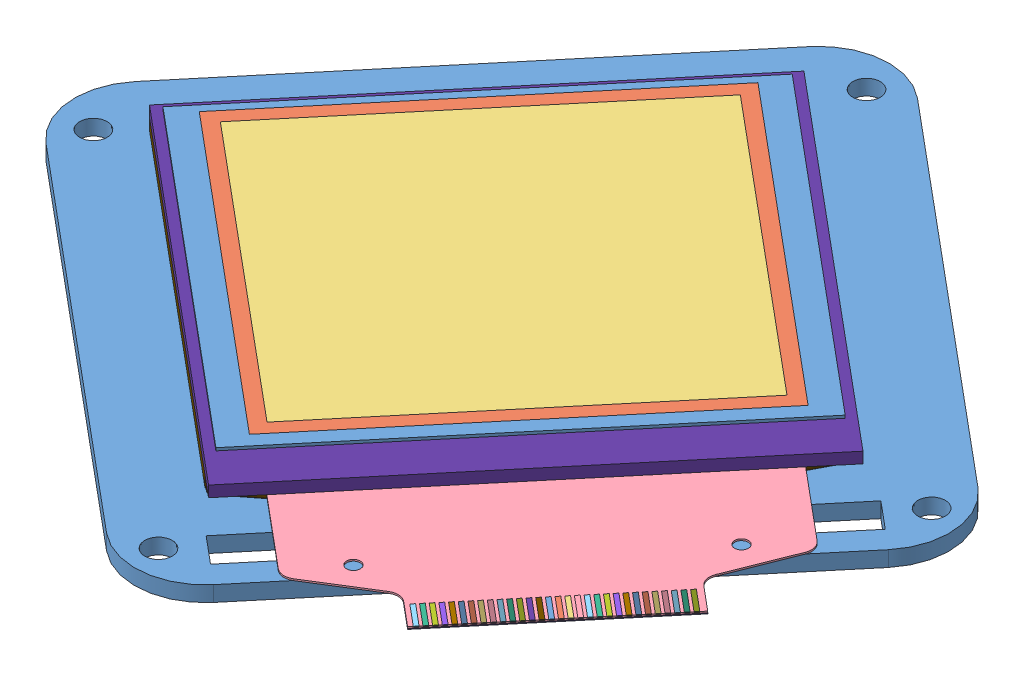
SolidWorks assembly main1, configuration 默认. Lengths in mm.
Overall size (158.53 67.75 132.39).
311 component instances, 75 part files, 5 mates.
Components (placement in the parent):
- case1-1: case1 [默认] at (23.4163 17.6612 38.5243) size (46 37.5 46)
- cubic1-1: cubic1 [默认] at (23.4663 19.1612 38.5743) x (0 0 1) z (-1 0 0) size (30 30 30)
- PCB_2020-12-27_16-28-50_2021-02-20_20-59-34-2: PCB_2020-12-27_16-28-50_2021-02-20_20-59-34 [默认] at (157.6255 16.5385 106.3075) x (-0.641097 0 0.76746) z (0 -1 0) size (45.01 51.47 7.58)
  - PCB_2020-12-27_16-28-50_2021-02-20_20-59-34.step-1: PCB_2020-12-27_16-28-50_2021-02-20_20-59-34.step [默认] at origin size (45.01 51.47 7.58)
    - Board.step-1: Board.step [默认] at origin size (45.01 45.01 1.12)
      - Open CASCADE STEP translator 6.8 3.1.1.step-1: Open CASCADE STEP translator 6.8 3.1.1.step [默认] at (0 0 -1.1227) size (45.01 45.01 1.12)
    - C34.step-1: C34.step [默认] at origin size (2.2 1.45 0.88)
      - c0805c101k5gactu.step-1: c0805c101k5gactu.step [默认] at (159.963 120.323 -10.6426) x (1 0 0) z (0 -1 0) size (2.2 0.88 1.45)
        - Open CASCADE STEP translator 6.8 3.2.1.1.step-1: Open CASCADE STEP translator 6.8 3.2.1.1.step [默认] at origin size (2 0.86 1.43)
        - Open CASCADE STEP translator 6.8 3.2.1.2.step-1: Open CASCADE STEP translator 6.8 3.2.1.2.step [默认] at origin size (0.34 0 0.18)
        - Open CASCADE STEP translator 6.8 3.2.1.3.step-1: Open CASCADE STEP translator 6.8 3.2.1.3.step [默认] at origin size (0.41 0 0.18)
        - Open CASCADE STEP translator 6.8 3.2.1.4.step-1: Open CASCADE STEP translator 6.8 3.2.1.4.step [默认] at origin size (0.21 0 0.18)
        - Open CASCADE STEP translator 6.8 3.2.1.5.step-1: Open CASCADE STEP translator 6.8 3.2.1.5.step [默认] at origin size (0.5 0.88 1.45)
        - Open CASCADE STEP translator 6.8 3.2.1.6.step-1: Open CASCADE STEP translator 6.8 3.2.1.6.step [默认] at origin size (0.5 0.88 1.45)
    - C14.step-1: C14.step [默认] at origin size (1.45 2.2 0.88)
      - c0805c101k5gactu.step-1: c0805c101k5gactu.step [默认] at (101.7169 -30.907 -10.6426) x (0 -1 0) z (-1 0 0) size (2.2 0.88 1.45)
        - Open CASCADE STEP translator 6.8 3.2.1.1.step-1: Open CASCADE STEP translator 6.8 3.2.1.1.step [默认] at origin size (2 0.86 1.43)
        - Open CASCADE STEP translator 6.8 3.2.1.2.step-1: Open CASCADE STEP translator 6.8 3.2.1.2.step [默认] at origin size (0.34 0 0.18)
        - Open CASCADE STEP translator 6.8 3.2.1.3.step-1: Open CASCADE STEP translator 6.8 3.2.1.3.step [默认] at origin size (0.41 0 0.18)
        - Open CASCADE STEP translator 6.8 3.2.1.4.step-1: Open CASCADE STEP translator 6.8 3.2.1.4.step [默认] at origin size (0.21 0 0.18)
        - Open CASCADE STEP translator 6.8 3.2.1.5.step-1: Open CASCADE STEP translator 6.8 3.2.1.5.step [默认] at origin size (0.5 0.88 1.45)
        - Open CASCADE STEP translator 6.8 3.2.1.6.step-1: Open CASCADE STEP translator 6.8 3.2.1.6.step [默认] at origin size (0.5 0.88 1.45)
    - C13.step-1: C13.step [默认] at origin size (0.95 1.77 0.95)
      - c0603x104k3ractu.step-1: c0603x104k3ractu.step [默认] at (16.3625 164.212 -10.6426) x (0 1 0) z (1 0 0) size (1.77 0.95 0.95)
        - Open CASCADE STEP translator 6.8 3.4.1.1.step-1: Open CASCADE STEP translator 6.8 3.4.1.1.step [默认] at origin size (1.57 0.93 0.93)
        - Open CASCADE STEP translator 6.8 3.4.1.2.step-1: Open CASCADE STEP translator 6.8 3.4.1.2.step [默认] at origin size (0.24 0 0.13)
        - Open CASCADE STEP translator 6.8 3.4.1.3.step-1: Open CASCADE STEP translator 6.8 3.4.1.3.step [默认] at origin size (0.29 0 0.13)
        - Open CASCADE STEP translator 6.8 3.4.1.4.step-1: Open CASCADE STEP translator 6.8 3.4.1.4.step [默认] at origin size (0.15 0 0.13)
        - Open CASCADE STEP translator 6.8 3.4.1.5.step-1: Open CASCADE STEP translator 6.8 3.4.1.5.step [默认] at origin size (0.45 0.95 0.95)
        - Open CASCADE STEP translator 6.8 3.4.1.6.step-1: Open CASCADE STEP translator 6.8 3.4.1.6.step [默认] at origin size (0.45 0.95 0.95)
    - C12.step-1: C12.step [默认] at origin size (0.95 1.77 0.95)
      - c0603x104k3ractu.step-1: c0603x104k3ractu.step [默认] at (9.3976 164.422 -10.6426) x (0 1 0) z (1 0 0) size (1.77 0.95 0.95)
        - Open CASCADE STEP translator 6.8 3.4.1.1.step-1: Open CASCADE STEP translator 6.8 3.4.1.1.step [默认] at origin size (1.57 0.93 0.93)
        - Open CASCADE STEP translator 6.8 3.4.1.2.step-1: Open CASCADE STEP translator 6.8 3.4.1.2.step [默认] at origin size (0.24 0 0.13)
        - Open CASCADE STEP translator 6.8 3.4.1.3.step-1: Open CASCADE STEP translator 6.8 3.4.1.3.step [默认] at origin size (0.29 0 0.13)
        - Open CASCADE STEP translator 6.8 3.4.1.4.step-1: Open CASCADE STEP translator 6.8 3.4.1.4.step [默认] at origin size (0.15 0 0.13)
        - Open CASCADE STEP translator 6.8 3.4.1.5.step-1: Open CASCADE STEP translator 6.8 3.4.1.5.step [默认] at origin size (0.45 0.95 0.95)
        - Open CASCADE STEP translator 6.8 3.4.1.6.step-1: Open CASCADE STEP translator 6.8 3.4.1.6.step [默认] at origin size (0.45 0.95 0.95)
    - USB2.step-1: USB2.step [默认] at origin size (5 7.8 2.7)
      - User_Library-micro_usb_SMD_RGB8421504.step-1: User_Library-micro_usb_SMD_RGB8421504.step [默认] at (44.3599 67.8551 1.27) x (0 -1 0) z (-1 0 0) size (7.8 2.7 5)
    - R7.step-1: R7.step [默认] at origin size (1.6 0.8 0.42)
      - User_Library-Res-0603.step-1: User_Library-Res-0603.step [默认] at (87.122 80.8989 0) x (-1 0 0) z (0 1 0) size (1.6 0.42 0.8)
    - L2.step-1: L2.step [默认] at origin size (0.86 1.6 0.51)
      - CircuitWorks-RESISTOR_0603.step-1: CircuitWorks-RESISTOR_0603.step [默认] at (61.595 79.7559 0) x (0 -1 0) z (-1 0 0) size (1.6 0.51 0.86)
    - P2.step-1: P2.step [默认] at origin size (20.43 5.11 2.05)
      - 3-1734839-0_RGB8421504.step-1: 3-1734839-0_RGB8421504.step [默认] at (66.548 57.4041 1.0414) x (1 0 0) z (0 -1 0) size (20.43 2.05 5.11)
    - D4.step-1: D4.step [默认] at origin size (3.7 1.6 1.27)
      - CircuitWorks-SOD123.step-1: CircuitWorks-SOD123.step [默认] at (72.4968 69.5129 0.0508) x (1 0 0) z (0 -1 0) size (3.7 1.27 1.6)
    - D5.step-1: D5.step [默认] at origin size (1.6 3.7 1.27)
      - CircuitWorks-SOD123.step-1: CircuitWorks-SOD123.step [默认] at (87.6301 64.8969 0.0508) x (0 1 0) z (1 0 0) size (3.7 1.27 1.6)
    - C21.step-1: C21.step [默认] at origin size (1.45 2.2 0.88)
      - c0805c101k5gactu.step-1: c0805c101k5gactu.step [默认] at (98.5419 -33.828 -10.6426) x (0 -1 0) z (-1 0 0) size (2.2 0.88 1.45)
        - Open CASCADE STEP translator 6.8 3.2.1.1.step-1: Open CASCADE STEP translator 6.8 3.2.1.1.step [默认] at origin size (2 0.86 1.43)
        - Open CASCADE STEP translator 6.8 3.2.1.2.step-1: Open CASCADE STEP translator 6.8 3.2.1.2.step [默认] at origin size (0.34 0 0.18)
        - Open CASCADE STEP translator 6.8 3.2.1.3.step-1: Open CASCADE STEP translator 6.8 3.2.1.3.step [默认] at origin size (0.41 0 0.18)
        - Open CASCADE STEP translator 6.8 3.2.1.4.step-1: Open CASCADE STEP translator 6.8 3.2.1.4.step [默认] at origin size (0.21 0 0.18)
        - Open CASCADE STEP translator 6.8 3.2.1.5.step-1: Open CASCADE STEP translator 6.8 3.2.1.5.step [默认] at origin size (0.5 0.88 1.45)
        - Open CASCADE STEP translator 6.8 3.2.1.6.step-1: Open CASCADE STEP translator 6.8 3.2.1.6.step [默认] at origin size (0.5 0.88 1.45)
    - C24.step-1: C24.step [默认] at origin size (1.45 2.2 0.88)
      - c0805c101k5gactu.step-1: c0805c101k5gactu.step [默认] at (2.51 156.471 -10.6426) x (0 1 0) z (1 0 0) size (2.2 0.88 1.45)
        - Open CASCADE STEP translator 6.8 3.2.1.1.step-1: Open CASCADE STEP translator 6.8 3.2.1.1.step [默认] at origin size (2 0.86 1.43)
        - Open CASCADE STEP translator 6.8 3.2.1.2.step-1: Open CASCADE STEP translator 6.8 3.2.1.2.step [默认] at origin size (0.34 0 0.18)
        - Open CASCADE STEP translator 6.8 3.2.1.3.step-1: Open CASCADE STEP translator 6.8 3.2.1.3.step [默认] at origin size (0.41 0 0.18)
        - Open CASCADE STEP translator 6.8 3.2.1.4.step-1: Open CASCADE STEP translator 6.8 3.2.1.4.step [默认] at origin size (0.21 0 0.18)
        - Open CASCADE STEP translator 6.8 3.2.1.5.step-1: Open CASCADE STEP translator 6.8 3.2.1.5.step [默认] at origin size (0.5 0.88 1.45)
        - Open CASCADE STEP translator 6.8 3.2.1.6.step-1: Open CASCADE STEP translator 6.8 3.2.1.6.step [默认] at origin size (0.5 0.88 1.45)
    - U7.step-1: U7.step [默认] at origin size (2.5 3 1.1)
      - CircuitWorks-SOT-23-5.step-1: CircuitWorks-SOT-23-5.step [默认] at (84.308 68.2431 -0.5131) x (0 1 0) z (1 0 0) size (3 1.1 2.5)
    - U5.step-1: U5.step [默认] at origin size (7 7 0.55)
      - User_Library-UFQFPN48.step-1: User_Library-UFQFPN48.step [默认] at (57.0029 73.1959 0) x (-1 0 0) z (0 0 1) size (7 7 0.55)
    - R13.step-1: R13.step [默认] at origin size (0.8 1.6 0.42)
      - User_Library-Res-0603.step-1: User_Library-Res-0603.step [默认] at (78.3388 65.957 0) x (0 1 0) z (1 0 0) size (1.6 0.42 0.8)
    - U4.step-1: U4.step [默认] at origin size (19.57 12.72 3.54)
      - User_Library-BK-885-TR.step-1: User_Library-BK-885-TR.step [默认] at (69.4691 84.328 0) x (1 0 0) z (0 -1 0) size (19.57 3.54 12.72)
    - U3.step-1: U3.step [默认] at origin size (0.8 1.6 0.42)
      - User_Library-Res-0603.step-1: User_Library-Res-0603.step [默认] at (61.3211 52.876 0) x (0 -1 0) z (-1 0 0) size (1.6 0.42 0.8)
    - C27.step-1: C27.step [默认] at origin size (0.95 1.77 0.95)
      - c0603x104k3ractu.step-1: c0603x104k3ractu.step [默认] at (123.9324 -30.647 -10.6426) x (0 -1 0) z (-1 0 0) size (1.77 0.95 0.95)
        - Open CASCADE STEP translator 6.8 3.4.1.1.step-1: Open CASCADE STEP translator 6.8 3.4.1.1.step [默认] at origin size (1.57 0.93 0.93)
        - Open CASCADE STEP translator 6.8 3.4.1.2.step-1: Open CASCADE STEP translator 6.8 3.4.1.2.step [默认] at origin size (0.24 0 0.13)
        - Open CASCADE STEP translator 6.8 3.4.1.3.step-1: Open CASCADE STEP translator 6.8 3.4.1.3.step [默认] at origin size (0.29 0 0.13)
        - Open CASCADE STEP translator 6.8 3.4.1.4.step-1: Open CASCADE STEP translator 6.8 3.4.1.4.step [默认] at origin size (0.15 0 0.13)
        - Open CASCADE STEP translator 6.8 3.4.1.5.step-1: Open CASCADE STEP translator 6.8 3.4.1.5.step [默认] at origin size (0.45 0.95 0.95)
        - Open CASCADE STEP translator 6.8 3.4.1.6.step-1: Open CASCADE STEP translator 6.8 3.4.1.6.step [默认] at origin size (0.45 0.95 0.95)
    - C20.step-1: C20.step [默认] at origin size (3.7 1.95 1.8)
      - c1206x223j2gacauto.step-1: c1206x223j2gacauto.step [默认] at (174.9253 96.5054 -10.6426) x (1 0 0) z (0 -1 0) size (3.7 1.8 1.95)
        - Open CASCADE STEP translator 6.8 3.20.1.1.step-1: Open CASCADE STEP translator 6.8 3.20.1.1.step [默认] at origin size (3.5 1.78 1.93)
        - Open CASCADE STEP translator 6.8 3.20.1.2.step-1: Open CASCADE STEP translator 6.8 3.20.1.2.step [默认] at origin size (0.7 0 0.37)
        - Open CASCADE STEP translator 6.8 3.20.1.3.step-1: Open CASCADE STEP translator 6.8 3.20.1.3.step [默认] at origin size (0.85 0 0.37)
        - Open CASCADE STEP translator 6.8 3.20.1.4.step-1: Open CASCADE STEP translator 6.8 3.20.1.4.step [默认] at origin size (0.44 0 0.37)
        - Open CASCADE STEP translator 6.8 3.20.1.5.step-1: Open CASCADE STEP translator 6.8 3.20.1.5.step [默认] at origin size (0.6 1.8 1.95)
        - Open CASCADE STEP translator 6.8 3.20.1.6.step-1: Open CASCADE STEP translator 6.8 3.20.1.6.step [默认] at origin size (0.6 1.8 1.95)
    - X3.step-1: X3.step [默认] at origin size (1.5 3.2 0.91)
      - crystal_rtf3215.step-1: crystal_rtf3215.step [默认] at (66.167 69.4691 0) x (0 1 0) z (1 0 0) size (3.2 0.91 1.5)
    - C28.step-1: C28.step [默认] at origin size (1.45 2.2 0.88)
      - c0805c101k5gactu.step-1: c0805c101k5gactu.step [默认] at (25.644 150.077 -10.6426) x (0 1 0) z (1 0 0) size (2.2 0.88 1.45)
        - Open CASCADE STEP translator 6.8 3.2.1.1.step-1: Open CASCADE STEP translator 6.8 3.2.1.1.step [默认] at origin size (2 0.86 1.43)
        - Open CASCADE STEP translator 6.8 3.2.1.2.step-1: Open CASCADE STEP translator 6.8 3.2.1.2.step [默认] at origin size (0.34 0 0.18)
        - Open CASCADE STEP translator 6.8 3.2.1.3.step-1: Open CASCADE STEP translator 6.8 3.2.1.3.step [默认] at origin size (0.41 0 0.18)
        - Open CASCADE STEP translator 6.8 3.2.1.4.step-1: Open CASCADE STEP translator 6.8 3.2.1.4.step [默认] at origin size (0.21 0 0.18)
        - Open CASCADE STEP translator 6.8 3.2.1.5.step-1: Open CASCADE STEP translator 6.8 3.2.1.5.step [默认] at origin size (0.5 0.88 1.45)
        - Open CASCADE STEP translator 6.8 3.2.1.6.step-1: Open CASCADE STEP translator 6.8 3.2.1.6.step [默认] at origin size (0.5 0.88 1.45)
    - C29.step-1: C29.step [默认] at origin size (1.45 2.2 0.88)
      - c0805c101k5gactu.step-1: c0805c101k5gactu.step [默认] at (102.7329 -43.6071 -10.6426) x (0 -1 0) z (-1 0 0) size (2.2 0.88 1.45)
        - Open CASCADE STEP translator 6.8 3.2.1.1.step-1: Open CASCADE STEP translator 6.8 3.2.1.1.step [默认] at origin size (2 0.86 1.43)
        - Open CASCADE STEP translator 6.8 3.2.1.2.step-1: Open CASCADE STEP translator 6.8 3.2.1.2.step [默认] at origin size (0.34 0 0.18)
        - Open CASCADE STEP translator 6.8 3.2.1.3.step-1: Open CASCADE STEP translator 6.8 3.2.1.3.step [默认] at origin size (0.41 0 0.18)
        - Open CASCADE STEP translator 6.8 3.2.1.4.step-1: Open CASCADE STEP translator 6.8 3.2.1.4.step [默认] at origin size (0.21 0 0.18)
        - Open CASCADE STEP translator 6.8 3.2.1.5.step-1: Open CASCADE STEP translator 6.8 3.2.1.5.step [默认] at origin size (0.5 0.88 1.45)
        - Open CASCADE STEP translator 6.8 3.2.1.6.step-1: Open CASCADE STEP translator 6.8 3.2.1.6.step [默认] at origin size (0.5 0.88 1.45)
    - C30.step-1: C30.step [默认] at origin size (1.45 2.2 0.88)
      - c0805c101k5gactu.step-1: c0805c101k5gactu.step [默认] at (97.9069 -43.6071 -10.6426) x (0 -1 0) z (-1 0 0) size (2.2 0.88 1.45)
        - Open CASCADE STEP translator 6.8 3.2.1.1.step-1: Open CASCADE STEP translator 6.8 3.2.1.1.step [默认] at origin size (2 0.86 1.43)
        - Open CASCADE STEP translator 6.8 3.2.1.2.step-1: Open CASCADE STEP translator 6.8 3.2.1.2.step [默认] at origin size (0.34 0 0.18)
        - Open CASCADE STEP translator 6.8 3.2.1.3.step-1: Open CASCADE STEP translator 6.8 3.2.1.3.step [默认] at origin size (0.41 0 0.18)
        - Open CASCADE STEP translator 6.8 3.2.1.4.step-1: Open CASCADE STEP translator 6.8 3.2.1.4.step [默认] at origin size (0.21 0 0.18)
        - Open CASCADE STEP translator 6.8 3.2.1.5.step-1: Open CASCADE STEP translator 6.8 3.2.1.5.step [默认] at origin size (0.5 0.88 1.45)
        - Open CASCADE STEP translator 6.8 3.2.1.6.step-1: Open CASCADE STEP translator 6.8 3.2.1.6.step [默认] at origin size (0.5 0.88 1.45)
    - U6.step-1: U6.step [默认] at origin size (2.5 3 1.1)
      - CircuitWorks-SOT-23-5.step-1: CircuitWorks-SOT-23-5.step [默认] at (52.8119 59.0989 -0.5131) x (0 -1 0) z (-1 0 0) size (3 1.1 2.5)
    - FPC1.step-1: FPC1.step [默认] at origin size (12.1 6.6 2)
      - 52746-1290_RGB10066329.step-1: 52746-1290_RGB10066329.step [默认] at (53.7211 87.5031 0) x (1 0 0) z (0 -1 0) size (12.1 2 6.6)
    - C18.step-1: C18.step [默认] at origin size (0.95 1.77 0.95)
      - c0603x104k3ractu.step-1: c0603x104k3ractu.step [默认] at (29.9716 149.69 -10.6426) x (0 1 0) z (1 0 0) size (1.77 0.95 0.95)
        - Open CASCADE STEP translator 6.8 3.4.1.1.step-1: Open CASCADE STEP translator 6.8 3.4.1.1.step [默认] at origin size (1.57 0.93 0.93)
        - Open CASCADE STEP translator 6.8 3.4.1.2.step-1: Open CASCADE STEP translator 6.8 3.4.1.2.step [默认] at origin size (0.24 0 0.13)
        - Open CASCADE STEP translator 6.8 3.4.1.3.step-1: Open CASCADE STEP translator 6.8 3.4.1.3.step [默认] at origin size (0.29 0 0.13)
        - Open CASCADE STEP translator 6.8 3.4.1.4.step-1: Open CASCADE STEP translator 6.8 3.4.1.4.step [默认] at origin size (0.15 0 0.13)
        - Open CASCADE STEP translator 6.8 3.4.1.5.step-1: Open CASCADE STEP translator 6.8 3.4.1.5.step [默认] at origin size (0.45 0.95 0.95)
        - Open CASCADE STEP translator 6.8 3.4.1.6.step-1: Open CASCADE STEP translator 6.8 3.4.1.6.step [默认] at origin size (0.45 0.95 0.95)
    - X1.step-1: X1.step [默认] at origin size (2.5 3.2 1.05)
      - User_Library-SMD-3225_4P.step-1: User_Library-SMD-3225_4P.step [默认] at (70.338 73.8309 0) x (0 -1 0) z (0 0 1) size (3.2 2.5 1.05)
    - C26.step-1: C26.step [默认] at origin size (2.2 1.45 0.88)
      - c0805c101k5gactu.step-1: c0805c101k5gactu.step [默认] at (183.605 114.818 -10.6426) x (1 0 0) z (0 -1 0) size (2.2 0.88 1.45)
        - Open CASCADE STEP translator 6.8 3.2.1.1.step-1: Open CASCADE STEP translator 6.8 3.2.1.1.step [默认] at origin size (2 0.86 1.43)
        - Open CASCADE STEP translator 6.8 3.2.1.2.step-1: Open CASCADE STEP translator 6.8 3.2.1.2.step [默认] at origin size (0.34 0 0.18)
        - Open CASCADE STEP translator 6.8 3.2.1.3.step-1: Open CASCADE STEP translator 6.8 3.2.1.3.step [默认] at origin size (0.41 0 0.18)
        - Open CASCADE STEP translator 6.8 3.2.1.4.step-1: Open CASCADE STEP translator 6.8 3.2.1.4.step [默认] at origin size (0.21 0 0.18)
        - Open CASCADE STEP translator 6.8 3.2.1.5.step-1: Open CASCADE STEP translator 6.8 3.2.1.5.step [默认] at origin size (0.5 0.88 1.45)
        - Open CASCADE STEP translator 6.8 3.2.1.6.step-1: Open CASCADE STEP translator 6.8 3.2.1.6.step [默认] at origin size (0.5 0.88 1.45)
    - C25.step-1: C25.step [默认] at origin size (1.45 2.2 0.88)
      - c0805c101k5gactu.step-1: c0805c101k5gactu.step [默认] at (36.439 156.681 -10.6426) x (0 1 0) z (1 0 0) size (2.2 0.88 1.45)
        - Open CASCADE STEP translator 6.8 3.2.1.1.step-1: Open CASCADE STEP translator 6.8 3.2.1.1.step [默认] at origin size (2 0.86 1.43)
        - Open CASCADE STEP translator 6.8 3.2.1.2.step-1: Open CASCADE STEP translator 6.8 3.2.1.2.step [默认] at origin size (0.34 0 0.18)
        - Open CASCADE STEP translator 6.8 3.2.1.3.step-1: Open CASCADE STEP translator 6.8 3.2.1.3.step [默认] at origin size (0.41 0 0.18)
        - Open CASCADE STEP translator 6.8 3.2.1.4.step-1: Open CASCADE STEP translator 6.8 3.2.1.4.step [默认] at origin size (0.21 0 0.18)
        - Open CASCADE STEP translator 6.8 3.2.1.5.step-1: Open CASCADE STEP translator 6.8 3.2.1.5.step [默认] at origin size (0.5 0.88 1.45)
        - Open CASCADE STEP translator 6.8 3.2.1.6.step-1: Open CASCADE STEP translator 6.8 3.2.1.6.step [默认] at origin size (0.5 0.88 1.45)
    - R17.step-1: R17.step [默认] at origin size (1.6 0.8 0.42)
      - User_Library-Res-0603.step-1: User_Library-Res-0603.step [默认] at (65.278 55.7531 0) x (1 0 0) z (0 -1 0) size (1.6 0.42 0.8)
    - R12.step-1: R12.step [默认] at origin size (0.8 1.6 0.42)
      - User_Library-Res-0603.step-1: User_Library-Res-0603.step [默认] at (63.2461 52.832 0) x (0 -1 0) z (-1 0 0) size (1.6 0.42 0.8)
    - R16.step-1: R16.step [默认] at origin size (1.6 0.8 0.42)
      - User_Library-Res-0603.step-1: User_Library-Res-0603.step [默认] at (62.103 55.7529 0) x (-1 0 0) z (0 1 0) size (1.6 0.42 0.8)
    - R15.step-1: R15.step [默认] at origin size (0.8 1.6 0.42)
      - User_Library-Res-0603.step-1: User_Library-Res-0603.step [默认] at (65.0241 52.832 0) x (0 -1 0) z (-1 0 0) size (1.6 0.42 0.8)
    - SW2.step-1: SW2.step [默认] at origin size (4.6 3.2 2.5)
      - skrpace010_RGB10066329.step-1: skrpace010_RGB10066329.step [默认] at (82.5499 81.661 0) x (-1 0 0) z (0 1 0) size (4.6 2.5 3.2)
    - SW1.step-1: SW1.step [默认] at origin size (4.6 3.2 2.5)
      - skrpace010_RGB10066329.step-1: skrpace010_RGB10066329.step [默认] at (82.4231 85.217 0) x (1 0 0) z (0 -1 0) size (4.6 2.5 3.2)
    - C17.step-1: C17.step [默认] at origin size (1.77 0.95 0.95)
      - c0603x104k3ractu.step-1: c0603x104k3ractu.step [默认] at (159.977 114.6814 -10.6426) x (1 0 0) z (0 -1 0) size (1.77 0.95 0.95)
        - Open CASCADE STEP translator 6.8 3.4.1.1.step-1: Open CASCADE STEP translator 6.8 3.4.1.1.step [默认] at origin size (1.57 0.93 0.93)
        - Open CASCADE STEP translator 6.8 3.4.1.2.step-1: Open CASCADE STEP translator 6.8 3.4.1.2.step [默认] at origin size (0.24 0 0.13)
        - Open CASCADE STEP translator 6.8 3.4.1.3.step-1: Open CASCADE STEP translator 6.8 3.4.1.3.step [默认] at origin size (0.29 0 0.13)
        - Open CASCADE STEP translator 6.8 3.4.1.4.step-1: Open CASCADE STEP translator 6.8 3.4.1.4.step [默认] at origin size (0.15 0 0.13)
        - Open CASCADE STEP translator 6.8 3.4.1.5.step-1: Open CASCADE STEP translator 6.8 3.4.1.5.step [默认] at origin size (0.45 0.95 0.95)
        - Open CASCADE STEP translator 6.8 3.4.1.6.step-1: Open CASCADE STEP translator 6.8 3.4.1.6.step [默认] at origin size (0.45 0.95 0.95)
    - C19.step-1: C19.step [默认] at origin size (1.77 0.95 0.95)
      - c0603x104k3ractu.step-1: c0603x104k3ractu.step [默认] at (159.977 112.0144 -10.6426) x (1 0 0) z (0 -1 0) size (1.77 0.95 0.95)
        - Open CASCADE STEP translator 6.8 3.4.1.1.step-1: Open CASCADE STEP translator 6.8 3.4.1.1.step [默认] at origin size (1.57 0.93 0.93)
        - Open CASCADE STEP translator 6.8 3.4.1.2.step-1: Open CASCADE STEP translator 6.8 3.4.1.2.step [默认] at origin size (0.24 0 0.13)
        - Open CASCADE STEP translator 6.8 3.4.1.3.step-1: Open CASCADE STEP translator 6.8 3.4.1.3.step [默认] at origin size (0.29 0 0.13)
        - Open CASCADE STEP translator 6.8 3.4.1.4.step-1: Open CASCADE STEP translator 6.8 3.4.1.4.step [默认] at origin size (0.15 0 0.13)
        - Open CASCADE STEP translator 6.8 3.4.1.5.step-1: Open CASCADE STEP translator 6.8 3.4.1.5.step [默认] at origin size (0.45 0.95 0.95)
        - Open CASCADE STEP translator 6.8 3.4.1.6.step-1: Open CASCADE STEP translator 6.8 3.4.1.6.step [默认] at origin size (0.45 0.95 0.95)
    - C16.step-1: C16.step [默认] at origin size (1.77 0.95 0.95)
      - c0603x104k3ractu.step-1: c0603x104k3ractu.step [默认] at (163.64 118.7894 -10.6426) x (1 0 0) z (0 -1 0) size (1.77 0.95 0.95)
        - Open CASCADE STEP translator 6.8 3.4.1.1.step-1: Open CASCADE STEP translator 6.8 3.4.1.1.step [默认] at origin size (1.57 0.93 0.93)
        - Open CASCADE STEP translator 6.8 3.4.1.2.step-1: Open CASCADE STEP translator 6.8 3.4.1.2.step [默认] at origin size (0.24 0 0.13)
        - Open CASCADE STEP translator 6.8 3.4.1.3.step-1: Open CASCADE STEP translator 6.8 3.4.1.3.step [默认] at origin size (0.29 0 0.13)
        - Open CASCADE STEP translator 6.8 3.4.1.4.step-1: Open CASCADE STEP translator 6.8 3.4.1.4.step [默认] at origin size (0.15 0 0.13)
        - Open CASCADE STEP translator 6.8 3.4.1.5.step-1: Open CASCADE STEP translator 6.8 3.4.1.5.step [默认] at origin size (0.45 0.95 0.95)
        - Open CASCADE STEP translator 6.8 3.4.1.6.step-1: Open CASCADE STEP translator 6.8 3.4.1.6.step [默认] at origin size (0.45 0.95 0.95)
    - C15.step-1: C15.step [默认] at origin size (1.77 0.95 0.95)
      - c0603x104k3ractu.step-1: c0603x104k3ractu.step [默认] at (163.64 116.5034 -10.6426) x (1 0 0) z (0 -1 0) size (1.77 0.95 0.95)
        - Open CASCADE STEP translator 6.8 3.4.1.1.step-1: Open CASCADE STEP translator 6.8 3.4.1.1.step [默认] at origin size (1.57 0.93 0.93)
        - Open CASCADE STEP translator 6.8 3.4.1.2.step-1: Open CASCADE STEP translator 6.8 3.4.1.2.step [默认] at origin size (0.24 0 0.13)
        - Open CASCADE STEP translator 6.8 3.4.1.3.step-1: Open CASCADE STEP translator 6.8 3.4.1.3.step [默认] at origin size (0.29 0 0.13)
        - Open CASCADE STEP translator 6.8 3.4.1.4.step-1: Open CASCADE STEP translator 6.8 3.4.1.4.step [默认] at origin size (0.15 0 0.13)
        - Open CASCADE STEP translator 6.8 3.4.1.5.step-1: Open CASCADE STEP translator 6.8 3.4.1.5.step [默认] at origin size (0.45 0.95 0.95)
        - Open CASCADE STEP translator 6.8 3.4.1.6.step-1: Open CASCADE STEP translator 6.8 3.4.1.6.step [默认] at origin size (0.45 0.95 0.95)
    - R14.step-1: R14.step [默认] at origin size (0.8 1.6 0.42)
      - User_Library-Res-0603.step-1: User_Library-Res-0603.step [默认] at (76.4338 65.957 0) x (0 1 0) z (1 0 0) size (1.6 0.42 0.8)
    - R11.step-1: R11.step [默认] at origin size (3.2 2.51 0.55)
      - User_Library-RESC3225X06N.step-1: User_Library-RESC3225X06N.step [默认] at (72.4971 66.592 0) size (3.2 2.51 0.55)
    - C23.step-1: C23.step [默认] at origin size (1.45 2.2 0.88)
      - c0805c101k5gactu.step-1: c0805c101k5gactu.step [默认] at (92.0649 -37.257 -10.6426) x (0 -1 0) z (-1 0 0) size (2.2 0.88 1.45)
        - Open CASCADE STEP translator 6.8 3.2.1.1.step-1: Open CASCADE STEP translator 6.8 3.2.1.1.step [默认] at origin size (2 0.86 1.43)
        - Open CASCADE STEP translator 6.8 3.2.1.2.step-1: Open CASCADE STEP translator 6.8 3.2.1.2.step [默认] at origin size (0.34 0 0.18)
        - Open CASCADE STEP translator 6.8 3.2.1.3.step-1: Open CASCADE STEP translator 6.8 3.2.1.3.step [默认] at origin size (0.41 0 0.18)
        - Open CASCADE STEP translator 6.8 3.2.1.4.step-1: Open CASCADE STEP translator 6.8 3.2.1.4.step [默认] at origin size (0.21 0 0.18)
        - Open CASCADE STEP translator 6.8 3.2.1.5.step-1: Open CASCADE STEP translator 6.8 3.2.1.5.step [默认] at origin size (0.5 0.88 1.45)
        - Open CASCADE STEP translator 6.8 3.2.1.6.step-1: Open CASCADE STEP translator 6.8 3.2.1.6.step [默认] at origin size (0.5 0.88 1.45)
    - C22.step-1: C22.step [默认] at origin size (1.45 2.2 0.88)
      - c0805c101k5gactu.step-1: c0805c101k5gactu.step [默认] at (96.0019 -33.828 -10.6426) x (0 -1 0) z (-1 0 0) size (2.2 0.88 1.45)
        - Open CASCADE STEP translator 6.8 3.2.1.1.step-1: Open CASCADE STEP translator 6.8 3.2.1.1.step [默认] at origin size (2 0.86 1.43)
        - Open CASCADE STEP translator 6.8 3.2.1.2.step-1: Open CASCADE STEP translator 6.8 3.2.1.2.step [默认] at origin size (0.34 0 0.18)
        - Open CASCADE STEP translator 6.8 3.2.1.3.step-1: Open CASCADE STEP translator 6.8 3.2.1.3.step [默认] at origin size (0.41 0 0.18)
        - Open CASCADE STEP translator 6.8 3.2.1.4.step-1: Open CASCADE STEP translator 6.8 3.2.1.4.step [默认] at origin size (0.21 0 0.18)
        - Open CASCADE STEP translator 6.8 3.2.1.5.step-1: Open CASCADE STEP translator 6.8 3.2.1.5.step [默认] at origin size (0.5 0.88 1.45)
        - Open CASCADE STEP translator 6.8 3.2.1.6.step-1: Open CASCADE STEP translator 6.8 3.2.1.6.step [默认] at origin size (0.5 0.88 1.45)
    - LED2.step-1: LED2.step [默认] at origin size (3.6 3.5 0.95)
      - User_Library-WS2813_3535.step-1: User_Library-WS2813_3535.step [默认] at (47.732 54.273 0) x (1 0 0) z (0 -1 0) size (3.6 0.95 3.5)
    - LED3.step-1: LED3.step [默认] at origin size (3.6 3.5 0.95)
      - User_Library-WS2813_3535.step-1: User_Library-WS2813_3535.step [默认] at (47.732 77.133 0) x (1 0 0) z (0 -1 0) size (3.6 0.95 3.5)
    - LED5.step-1: LED5.step [默认] at origin size (3.6 3.5 0.95)
      - User_Library-WS2813_3535.step-1: User_Library-WS2813_3535.step [默认] at (85.324 54.273 0) x (1 0 0) z (0 -1 0) size (3.6 0.95 3.5)
    - LED4.step-1: LED4.step [默认] at origin size (3.6 3.5 0.95)
      - User_Library-WS2813_3535.step-1: User_Library-WS2813_3535.step [默认] at (85.324 77.133 0) x (1 0 0) z (0 -1 0) size (3.6 0.95 3.5)
    - C31.step-1: C31.step [默认] at origin size (1.45 2.2 0.88)
      - c0805c101k5gactu.step-1: c0805c101k5gactu.step [默认] at (115.199 -43.651 -10.6426) x (0 -1 0) z (-1 0 0) size (2.2 0.88 1.45)
        - Open CASCADE STEP translator 6.8 3.2.1.1.step-1: Open CASCADE STEP translator 6.8 3.2.1.1.step [默认] at origin size (2 0.86 1.43)
        - Open CASCADE STEP translator 6.8 3.2.1.2.step-1: Open CASCADE STEP translator 6.8 3.2.1.2.step [默认] at origin size (0.34 0 0.18)
        - Open CASCADE STEP translator 6.8 3.2.1.3.step-1: Open CASCADE STEP translator 6.8 3.2.1.3.step [默认] at origin size (0.41 0 0.18)
        - Open CASCADE STEP translator 6.8 3.2.1.4.step-1: Open CASCADE STEP translator 6.8 3.2.1.4.step [默认] at origin size (0.21 0 0.18)
        - Open CASCADE STEP translator 6.8 3.2.1.5.step-1: Open CASCADE STEP translator 6.8 3.2.1.5.step [默认] at origin size (0.5 0.88 1.45)
        - Open CASCADE STEP translator 6.8 3.2.1.6.step-1: Open CASCADE STEP translator 6.8 3.2.1.6.step [默认] at origin size (0.5 0.88 1.45)
    - C32.step-1: C32.step [默认] at origin size (1.45 2.2 0.88)
      - c0805c101k5gactu.step-1: c0805c101k5gactu.step [默认] at (13.178 150.121 -10.6426) x (0 1 0) z (1 0 0) size (2.2 0.88 1.45)
        - Open CASCADE STEP translator 6.8 3.2.1.1.step-1: Open CASCADE STEP translator 6.8 3.2.1.1.step [默认] at origin size (2 0.86 1.43)
        - Open CASCADE STEP translator 6.8 3.2.1.2.step-1: Open CASCADE STEP translator 6.8 3.2.1.2.step [默认] at origin size (0.34 0 0.18)
        - Open CASCADE STEP translator 6.8 3.2.1.3.step-1: Open CASCADE STEP translator 6.8 3.2.1.3.step [默认] at origin size (0.41 0 0.18)
        - Open CASCADE STEP translator 6.8 3.2.1.4.step-1: Open CASCADE STEP translator 6.8 3.2.1.4.step [默认] at origin size (0.21 0 0.18)
        - Open CASCADE STEP translator 6.8 3.2.1.5.step-1: Open CASCADE STEP translator 6.8 3.2.1.5.step [默认] at origin size (0.5 0.88 1.45)
        - Open CASCADE STEP translator 6.8 3.2.1.6.step-1: Open CASCADE STEP translator 6.8 3.2.1.6.step [默认] at origin size (0.5 0.88 1.45)
    - CN9.step-1: CN9.step [默认] at origin size (4.85 8.25 4.35)
      - User_Library-SM04B-GHS-TB_RGB14277081.step-1: User_Library-SM04B-GHS-TB_RGB14277081.step [默认] at (76.448 78.464 0) x (0 1 0) z (1 0 0) size (8.25 4.35 4.85)
    - C35.step-1: C35.step [默认] at origin size (1.77 0.95 0.95)
      - c0603x104k3ractu.step-1: c0603x104k3ractu.step [默认] at (-9.482 38.9886 -10.6426) x (-1 0 0) z (0 1 0) size (1.77 0.95 0.95)
        - Open CASCADE STEP translator 6.8 3.4.1.1.step-1: Open CASCADE STEP translator 6.8 3.4.1.1.step [默认] at origin size (1.57 0.93 0.93)
        - Open CASCADE STEP translator 6.8 3.4.1.2.step-1: Open CASCADE STEP translator 6.8 3.4.1.2.step [默认] at origin size (0.24 0 0.13)
        - Open CASCADE STEP translator 6.8 3.4.1.3.step-1: Open CASCADE STEP translator 6.8 3.4.1.3.step [默认] at origin size (0.29 0 0.13)
        - Open CASCADE STEP translator 6.8 3.4.1.4.step-1: Open CASCADE STEP translator 6.8 3.4.1.4.step [默认] at origin size (0.15 0 0.13)
        - Open CASCADE STEP translator 6.8 3.4.1.5.step-1: Open CASCADE STEP translator 6.8 3.4.1.5.step [默认] at origin size (0.45 0.95 0.95)
        - Open CASCADE STEP translator 6.8 3.4.1.6.step-1: Open CASCADE STEP translator 6.8 3.4.1.6.step [默认] at origin size (0.45 0.95 0.95)
    - C11.step-1: C11.step [默认] at origin size (1.77 0.95 0.95)
      - c0603x104k3ractu.step-1: c0603x104k3ractu.step [默认] at (149.436 121.6664 -10.6426) x (1 0 0) z (0 -1 0) size (1.77 0.95 0.95)
        - Open CASCADE STEP translator 6.8 3.4.1.1.step-1: Open CASCADE STEP translator 6.8 3.4.1.1.step [默认] at origin size (1.57 0.93 0.93)
        - Open CASCADE STEP translator 6.8 3.4.1.2.step-1: Open CASCADE STEP translator 6.8 3.4.1.2.step [默认] at origin size (0.24 0 0.13)
        - Open CASCADE STEP translator 6.8 3.4.1.3.step-1: Open CASCADE STEP translator 6.8 3.4.1.3.step [默认] at origin size (0.29 0 0.13)
        - Open CASCADE STEP translator 6.8 3.4.1.4.step-1: Open CASCADE STEP translator 6.8 3.4.1.4.step [默认] at origin size (0.15 0 0.13)
        - Open CASCADE STEP translator 6.8 3.4.1.5.step-1: Open CASCADE STEP translator 6.8 3.4.1.5.step [默认] at origin size (0.45 0.95 0.95)
        - Open CASCADE STEP translator 6.8 3.4.1.6.step-1: Open CASCADE STEP translator 6.8 3.4.1.6.step [默认] at origin size (0.45 0.95 0.95)
    - C36.step-1: C36.step [默认] at origin size (2.2 1.45 0.88)
      - c0805c101k5gactu.step-1: c0805c101k5gactu.step [默认] at (-43.651 36.312 -10.6426) x (-1 0 0) z (0 1 0) size (2.2 0.88 1.45)
        - Open CASCADE STEP translator 6.8 3.2.1.1.step-1: Open CASCADE STEP translator 6.8 3.2.1.1.step [默认] at origin size (2 0.86 1.43)
        - Open CASCADE STEP translator 6.8 3.2.1.2.step-1: Open CASCADE STEP translator 6.8 3.2.1.2.step [默认] at origin size (0.34 0 0.18)
        - Open CASCADE STEP translator 6.8 3.2.1.3.step-1: Open CASCADE STEP translator 6.8 3.2.1.3.step [默认] at origin size (0.41 0 0.18)
        - Open CASCADE STEP translator 6.8 3.2.1.4.step-1: Open CASCADE STEP translator 6.8 3.2.1.4.step [默认] at origin size (0.21 0 0.18)
        - Open CASCADE STEP translator 6.8 3.2.1.5.step-1: Open CASCADE STEP translator 6.8 3.2.1.5.step [默认] at origin size (0.5 0.88 1.45)
        - Open CASCADE STEP translator 6.8 3.2.1.6.step-1: Open CASCADE STEP translator 6.8 3.2.1.6.step [默认] at origin size (0.5 0.88 1.45)
    - C33.step-1: C33.step [默认] at origin size (1.77 0.95 0.95)
      - c0603x104k3ractu.step-1: c0603x104k3ractu.step [默认] at (-32.743 30.9046 -10.6426) x (-1 0 0) z (0 1 0) size (1.77 0.95 0.95)
        - Open CASCADE STEP translator 6.8 3.4.1.1.step-1: Open CASCADE STEP translator 6.8 3.4.1.1.step [默认] at origin size (1.57 0.93 0.93)
        - Open CASCADE STEP translator 6.8 3.4.1.2.step-1: Open CASCADE STEP translator 6.8 3.4.1.2.step [默认] at origin size (0.24 0 0.13)
        - Open CASCADE STEP translator 6.8 3.4.1.3.step-1: Open CASCADE STEP translator 6.8 3.4.1.3.step [默认] at origin size (0.29 0 0.13)
        - Open CASCADE STEP translator 6.8 3.4.1.4.step-1: Open CASCADE STEP translator 6.8 3.4.1.4.step [默认] at origin size (0.15 0 0.13)
        - Open CASCADE STEP translator 6.8 3.4.1.5.step-1: Open CASCADE STEP translator 6.8 3.4.1.5.step [默认] at origin size (0.45 0.95 0.95)
        - Open CASCADE STEP translator 6.8 3.4.1.6.step-1: Open CASCADE STEP translator 6.8 3.4.1.6.step [默认] at origin size (0.45 0.95 0.95)
    - Free-Models.step-1: Free-Models.step [默认] at origin size (33.8 46.35 1.8)
      - mcot128128az-rgbm.step-1: mcot128128az-rgbm.step [默认] at (83.7239 85.5761 -3.1293) x (-1 0 0) z (0 0 -1) size (33.8 46.35 1.8)
        - Open CASCADE STEP translator 6.8 3.56.1.1.step-1: Open CASCADE STEP translator 6.8 3.56.1.1.step [默认] at origin size (33.8 34 0.8)
        - Open CASCADE STEP translator 6.8 3.56.1.2.step-1: Open CASCADE STEP translator 6.8 3.56.1.2.step [默认] at origin size (33.8 32 0.8)
        - Open CASCADE STEP translator 6.8 3.56.1.3.step-1: Open CASCADE STEP translator 6.8 3.56.1.3.step [默认] at origin size (32.5 30.5 0.2)
        - Open CASCADE STEP translator 6.8 3.56.1.4.step-1: Open CASCADE STEP translator 6.8 3.56.1.4.step [默认] at origin size (28.86 28.86 0.1)
        - Open CASCADE STEP translator 6.8 3.56.1.5.step-1: Open CASCADE STEP translator 6.8 3.56.1.5.step [默认] at origin size (26.86 26.86 0.05)
        - Open CASCADE STEP translator 6.8 3.56.1.6.step-1: Open CASCADE STEP translator 6.8 3.56.1.6.step [默认] at origin size (27.83 14.35 0.12)
        - Open CASCADE STEP translator 6.8 3.56.1.7.step-1: Open CASCADE STEP translator 6.8 3.56.1.7.step [默认] at origin size (0.3 2 0.06)
        - Open CASCADE STEP translator 6.8 3.56.1.8.step-1: Open CASCADE STEP translator 6.8 3.56.1.8.step [默认] at origin size (0.3 2 0.06)
        - Open CASCADE STEP translator 6.8 3.56.1.9.step-1: Open CASCADE STEP translator 6.8 3.56.1.9.step [默认] at origin size (0.3 2 0.06)
        - Open CASCADE STEP translator 6.8 3.56.1.10.step-1: Open CASCADE STEP translator 6.8 3.56.1.10.step [默认] at origin size (0.3 2 0.06)
        - Open CASCADE STEP translator 6.8 3.56.1.11.step-1: Open CASCADE STEP translator 6.8 3.56.1.11.step [默认] at origin size (0.3 2 0.06)
        - Open CASCADE STEP translator 6.8 3.56.1.12.step-1: Open CASCADE STEP translator 6.8 3.56.1.12.step [默认] at origin size (0.3 2 0.06)
        - Open CASCADE STEP translator 6.8 3.56.1.13.step-1: Open CASCADE STEP translator 6.8 3.56.1.13.step [默认] at origin size (0.3 2 0.06)
        - Open CASCADE STEP translator 6.8 3.56.1.14.step-1: Open CASCADE STEP translator 6.8 3.56.1.14.step [默认] at origin size (0.3 2 0.06)
        - Open CASCADE STEP translator 6.8 3.56.1.15.step-1: Open CASCADE STEP translator 6.8 3.56.1.15.step [默认] at origin size (0.3 2 0.06)
        - Open CASCADE STEP translator 6.8 3.56.1.16.step-1: Open CASCADE STEP translator 6.8 3.56.1.16.step [默认] at origin size (0.3 2 0.06)
        - Open CASCADE STEP translator 6.8 3.56.1.17.step-1: Open CASCADE STEP translator 6.8 3.56.1.17.step [默认] at origin size (0.3 2 0.06)
        - Open CASCADE STEP translator 6.8 3.56.1.18.step-1: Open CASCADE STEP translator 6.8 3.56.1.18.step [默认] at origin size (0.3 2 0.06)
        - Open CASCADE STEP translator 6.8 3.56.1.19.step-1: Open CASCADE STEP translator 6.8 3.56.1.19.step [默认] at origin size (0.3 2 0.06)
        - Open CASCADE STEP translator 6.8 3.56.1.20.step-1: Open CASCADE STEP translator 6.8 3.56.1.20.step [默认] at origin size (0.3 2 0.06)
        - Open CASCADE STEP translator 6.8 3.56.1.21.step-1: Open CASCADE STEP translator 6.8 3.56.1.21.step [默认] at origin size (0.3 2 0.06)
        - Open CASCADE STEP translator 6.8 3.56.1.22.step-1: Open CASCADE STEP translator 6.8 3.56.1.22.step [默认] at origin size (0.3 2 0.06)
        - Open CASCADE STEP translator 6.8 3.56.1.23.step-1: Open CASCADE STEP translator 6.8 3.56.1.23.step [默认] at origin size (0.3 2 0.06)
        - Open CASCADE STEP translator 6.8 3.56.1.24.step-1: Open CASCADE STEP translator 6.8 3.56.1.24.step [默认] at origin size (0.3 2 0.06)
        - Open CASCADE STEP translator 6.8 3.56.1.25.step-1: Open CASCADE STEP translator 6.8 3.56.1.25.step [默认] at origin size (0.3 2 0.06)
        - Open CASCADE STEP translator 6.8 3.56.1.26.step-1: Open CASCADE STEP translator 6.8 3.56.1.26.step [默认] at origin size (0.3 2 0.06)
        - Open CASCADE STEP translator 6.8 3.56.1.27.step-1: Open CASCADE STEP translator 6.8 3.56.1.27.step [默认] at origin size (0.3 2 0.06)
        - Open CASCADE STEP translator 6.8 3.56.1.28.step-1: Open CASCADE STEP translator 6.8 3.56.1.28.step [默认] at origin size (0.3 2 0.06)
        - Open CASCADE STEP translator 6.8 3.56.1.29.step-1: Open CASCADE STEP translator 6.8 3.56.1.29.step [默认] at origin size (0.3 2 0.06)
        - Open CASCADE STEP translator 6.8 3.56.1.30.step-1: Open CASCADE STEP translator 6.8 3.56.1.30.step [默认] at origin size (0.3 2 0.06)
        - Open CASCADE STEP translator 6.8 3.56.1.31.step-1: Open CASCADE STEP translator 6.8 3.56.1.31.step [默认] at origin size (0.3 2 0.06)
        - Open CASCADE STEP translator 6.8 3.56.1.32.step-1: Open CASCADE STEP translator 6.8 3.56.1.32.step [默认] at origin size (0.3 2 0.06)
        - Open CASCADE STEP translator 6.8 3.56.1.33.step-1: Open CASCADE STEP translator 6.8 3.56.1.33.step [默认] at origin size (0.3 2 0.06)
        - Open CASCADE STEP translator 6.8 3.56.1.34.step-1: Open CASCADE STEP translator 6.8 3.56.1.34.step [默认] at origin size (0.3 2 0.06)
        - Open CASCADE STEP translator 6.8 3.56.1.35.step-1: Open CASCADE STEP translator 6.8 3.56.1.35.step [默认] at origin size (0.3 2 0.06)
        - Open CASCADE STEP translator 6.8 3.56.1.36.step-1: Open CASCADE STEP translator 6.8 3.56.1.36.step [默认] at origin size (0.3 2 0.06)
        - Open CASCADE STEP translator 6.8 3.56.1.37.step-1: Open CASCADE STEP translator 6.8 3.56.1.37.step [默认] at origin size (15.51 3 0.06)
        - Open CASCADE STEP translator 6.8 3.56.1.38.step-1: Open CASCADE STEP translator 6.8 3.56.1.38.step [默认] at origin size (33.8 2 0.8)
- stand1-1: stand1 [默认] at (-37.5136 11.5385 74.5499) x (0.001816 0 0.999998) z (-0.999998 0 0.001816) size (61.5 29.73 48)
Mates (geometry in assembly coordinates):
- 重合27: coincident anti-aligned: plane of case1-1 through (5.9163 17.6612 21.0243) normal (0 -1 0); plane of PCB_2020-12-27_16-28-50_2021-02-20_20-59-34-2/PCB_2020-12-27_16-28-50_2021-02-20_20-59-34.step-1/Board.step-1/Open CASCADE STEP translator 6.8 3.1.1.step-1 through (90.5227 17.6612 107.6751) normal (0 1 0)
- 重合28: coincident anti-aligned: plane of case1-1 through (23.4163 49.1612 38.5243) normal (0 -1 0); plane of cubic1-1 through (23.4663 49.1612 38.5743) normal (0 1 0)
- 重合29: coincident anti-aligned: plane of case1-1 through (8.3663 49.1612 53.5743) normal (0 0 -1); plane of cubic1-1 through (38.4663 49.1612 53.5743) normal (0 0 1)
- 重合30: coincident anti-aligned: plane of case1-1 through (38.4663 49.1612 23.4743) normal (-1 0 0); plane of cubic1-1 through (38.4663 49.1612 23.5743) normal (1 0 0)
- 重合31: coincident anti-aligned: plane of PCB_2020-12-27_16-28-50_2021-02-20_20-59-34-2/PCB_2020-12-27_16-28-50_2021-02-20_20-59-34.step-1/Board.step-1/Open CASCADE STEP translator 6.8 3.1.1.step-1 through (90.5227 16.5385 107.6751) normal (0 -1 0); plane of stand1-1 through (-37.5136 16.5385 74.5499) normal (0 1 0)
